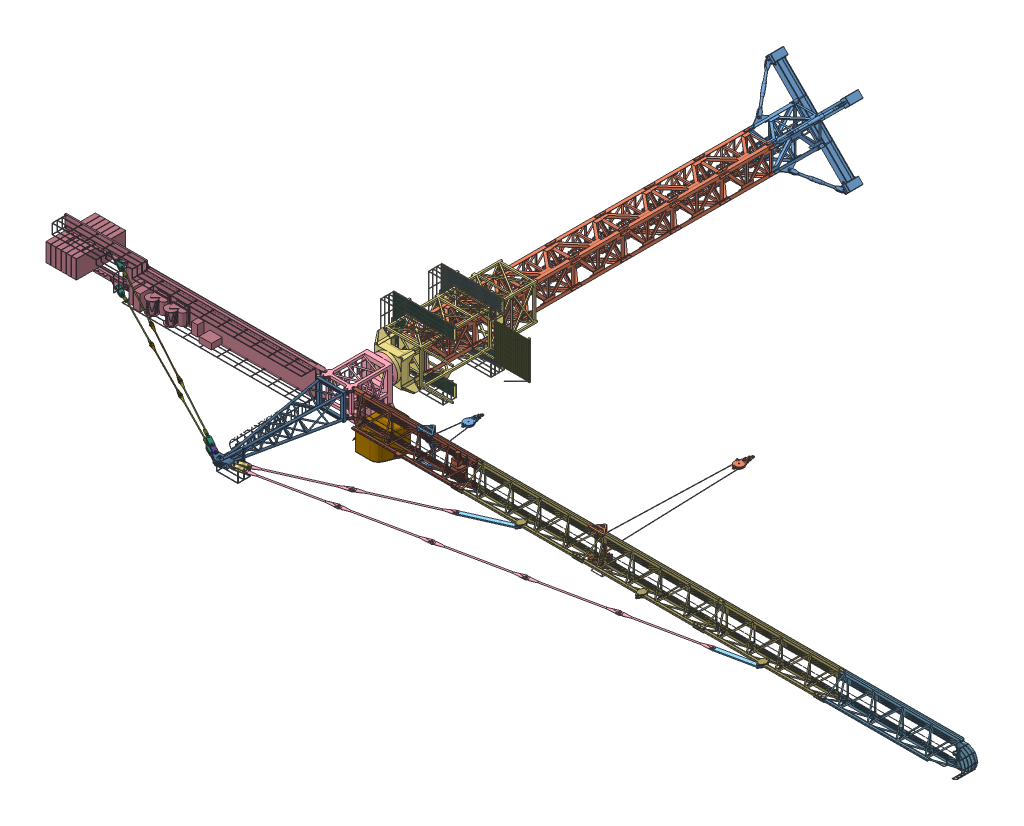
SolidWorks assembly ASS crane, configuration Default. Lengths in mm.
Overall size (55095.39 5209.24 36556.54).
50 component instances, 23 part files, 0 mates.
Components (placement in the parent):
- ASS crane.stp-1: ASS crane.stp [Default] at origin size (55095.39 5209.24 36556.54)
  - crane body segment ground base.stp-1: crane body segment ground base.stp [Default] at origin size (5118.48 5118.48 3780)
  - crane body segment.stp-1: crane body segment.stp [Default] at (0 0 3000) size (1820 1820 3425)
  - crane body segment.stp-2: crane body segment.stp [Default] at (0 0 6000) size (1820 1820 3425)
  - crane body segment.stp-3: crane body segment.stp [Default] at (0 0 9000) size (1820 1820 3425)
  - crane body segment.stp-4: crane body segment.stp [Default] at (0 0 12000) size (1820 1820 3425)
  - crane body segment.stp-5: crane body segment.stp [Default] at (0 0 15000) size (1820 1820 3425)
  - crane body segment.stp-6: crane body segment.stp [Default] at (0 0 18000) size (1820 1820 3425)
  - crane body segment.stp-7: crane body segment.stp [Default] at (0 0 21000) size (1820 1820 3425)
  - crane climbing segment.stp-1: crane climbing segment.stp [Default] at (0 0 19033.3333) size (5950 3705.69 8170)
  - crane cabin segment.stp-1: crane cabin segment.stp [Default] at (0 0 19178.3333) size (2700 3325 3075)
  - crane body segment top plates.stp-1: crane body segment top plates.stp [Default] at (-100 0 15733.3333) size (3655.69 3655.69 10)
  - crane body segment top plates - opened.stp-1: crane body segment top plates - opened.stp [Default] at (-100 0 18633.3333) size (3655.69 3655.69 458.61)
  - crane body segment top plates2.stp-1: crane body segment top plates2.stp [Default] at (0 0 18633.3333) size (2100 2205.69 10)
  - motor.stp-1: motor.stp [Default] at (1173.0769 -182.9762 26585.7508) size (400 387.98 900)
  - cabin.stp-1: cabin.stp [Default] at (25 125 19528.3333) size (2001.66 1500 2050)
  - apex.stp-1: apex.stp [Default] at (0 0 19378.3333) size (1983.62 1737.73 7223.21)
  - crane jib - base.stp-1: crane jib - base.stp [Default] at (0 0 -4621.6667) size (8040 1822.44 1872.95)
  - crane jib main.stp-1: crane jib main.stp [Default] at (7315 0 -4621.6667) size (7665 1600 1855.45)
  - crane jib main.stp-2: crane jib main.stp [Default] at (14630 0 -4621.6667) size (7665 1600 1855.45)
  - crane jib main.stp-3: crane jib main.stp [Default] at (21945 0 -4621.6667) size (7665 1600 1855.45)
  - counter weight segment.stp-1: counter weight segment.stp [Default] at (1600 1600 -4621.6667) x (-1 0 0) z (0 0 1) size (15690.39 2165 3000)
  - crane jib last.stp-1: crane jib last.stp [Default] at (29260 0 -4621.6667) size (8200.04 1600 1682.44)
  - rear pendant counterjib conector.stp-1: rear pendant counterjib conector.stp [Default] at (-12175 165 28787.7078) x (0.88476 0 0.466047) z (0.466047 0 -0.88476) size (740 220 240)
  - rear pendant counterjib conector.stp-2: rear pendant counterjib conector.stp [Default] at (-12175 1435 28787.7078) x (0.88476 0 0.466047) z (-0.466047 0 0.88476) size (740 220 240)
  - rear cable.stp-1: rear cable.stp [Default] at (-11723.8181 1472.1276 29025.3679) x (-0.031767 -0.999355 -0.016733) z (-0.466047 0 0.88476) size (120.1 4384.6 229.62)
  - rear cable.stp-2: rear cable.stp [Default] at (-11723.8181 127.8724 29025.3679) x (0.031767 -0.999355 0.016733) z (-0.466047 0 0.88476) size (120.1 4384.6 229.62)
  - apex rear conector.stp-1: apex rear conector.stp [Default] at (19.0206 650 35210.9097) x (-0.038593 0.999048 -0.020329) z (-0.466047 0 0.88476) size (95.83 739.19 240)
  - apex rear conector.stp-2: apex rear conector.stp [Default] at (19.0206 950 35210.9097) x (-0.038593 -0.999048 -0.020329) z (0.466047 0 -0.88476) size (95.83 739.19 240)
  - rear pendant counterjib conector.stp-3: rear pendant counterjib conector.stp [Default] at (-201.9588 960.9048 35094.5087) x (-0.883918 0.043619 -0.465604) z (0.466047 0 -0.88476) size (740 220 240)
  - rear pendant counterjib conector.stp-4: rear pendant counterjib conector.stp [Default] at (-198.8714 559.1713 35096.135) x (-0.883918 -0.043619 -0.465604) z (0.466047 0 -0.88476) size (740 220 240)
  - rear cable.stp-3: rear cable.stp [Default] at (-651.2349 1022.4955 34857.8525) x (0.031767 0.999355 0.016733) z (-0.466047 0 0.88476) size (120.1 4384.6 229.62)
  - rear cable.stp-4: rear cable.stp [Default] at (-651.2349 577.5045 34857.8525) x (-0.031767 0.999355 -0.016733) z (-0.466047 0 0.88476) size (120.1 4384.6 229.62)
  - cable conector.stp-1: cable conector.stp [Default] at (-6198.8594 351.3766 31884.7794) x (-0.031767 0.999355 -0.016733) z (-0.466047 0 0.88476) size (198.88 4355.94 190.95)
  - cable conector.stp-2: cable conector.stp [Default] at (-6198.8594 1248.6234 31884.7794) x (0.031767 0.999355 0.016733) z (-0.466047 0 0.88476) size (198.88 4355.94 190.95)
  - trolley sc.stp-1: trolley sc.stp [Default] at (3862.0611 0 -4618.4821) x (0.999999 0 -0.001227) z (0.001227 0 0.999999) size (1438.92 1790 3638.61)
  - trolley.stp-1: trolley.stp [Default] at (14262.069 0 -4618.4821) x (0.999999 0 -0.001227) z (0.001227 0 0.999999) size (1438.92 2302 9638.61)
  - fore cable conector.stp-1: fore cable conector.stp [Default] at (1889.585 840 35251.0244) x (-0.97917 0 0.203042) z (0.203042 0 0.97917) size (740 210 240)
  - fore cable conector.stp-2: fore cable conector.stp [Default] at (1811.8924 840 34893.7306) x (-0.914082 0 0.40553) z (0.40553 0 0.914082) size (740 210 240)
  - fore cable.stp-1: fore cable.stp [Default] at (3969.1253 800 33936.6799) x (0.914082 0 -0.40553) z (-0.40553 0 -0.914082) size (5000 222.08 202.07)
  - fore cable.stp-2: fore cable.stp [Default] at (8356.7177 800 31990.1362) x (0.914082 0 -0.40553) z (-0.40553 0 -0.914082) size (5000 222.08 202.07)
  - fore cable.stp-3: fore cable.stp [Default] at (4278.7596 800 34755.6009) x (0.97917 0 -0.203042) z (0.203042 0 0.97917) size (5000 222.08 202.07)
  - fore cable.stp-4: fore cable.stp [Default] at (8978.7754 800 33780.9973) x (0.97917 0 -0.203042) z (0.203042 0 0.97917) size (5000 222.08 202.07)
  - fore cable.stp-5: fore cable.stp [Default] at (13678.7911 800 32806.3937) x (0.97917 0 -0.203042) z (0.203042 0 0.97917) size (5000 222.08 202.07)
  - fore cable.stp-6: fore cable.stp [Default] at (18378.8068 800 31831.7901) x (0.97917 0 -0.203042) z (0.203042 0 0.97917) size (5000 222.08 202.07)
  - fore cable.stp-7: fore cable.stp [Default] at (23078.8225 800 30857.1864) x (0.97917 0 -0.203042) z (0.203042 0 0.97917) size (5000 222.08 202.07)
  - fore jib connector.stp-1: fore jib connector.stp [Default] at (12378.6774 800 30205.8044) x (0.914082 0 -0.40553) z (0.40553 0 0.914082) size (2120 70 240)
  - fore jib connector.stp-2: fore jib connector.stp [Default] at (11242.5563 800 30709.8415) x (-0.914082 0 0.40553) z (-0.40553 0 -0.914082) size (2120 70 240)
  - fore jib connector.stp-3: fore jib connector.stp [Default] at (27387.1703 800 29963.7998) x (0.97917 0 -0.203042) z (0.203042 0 0.97917) size (2120 70 240)
  - fore jib connector.stp-4: fore jib connector.stp [Default] at (25742.3799 800 30304.8664) x (-0.97917 0 0.203042) z (-0.203042 0 -0.97917) size (2120 70 240)
